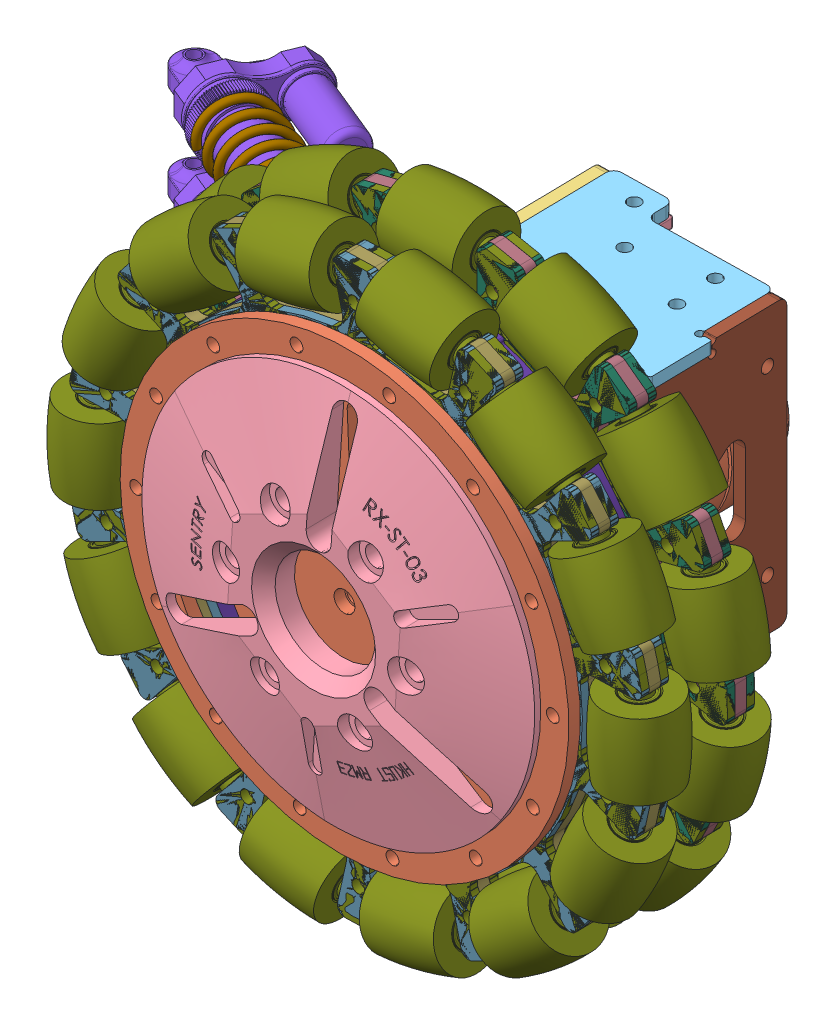
SolidWorks assembly 1.5GEN_sentry_suspension_module, configuration Default. Lengths in mm.
Overall size (247.79 229.92 117.48).
42 component instances, 23 part files, 105 mates.
Components (placement in the parent):
- 3508_standard_motor_mount1-1: 3508_standard_motor_mount1 [Default] at (120.0122 35.5003 50.6966) x (0.999831 0 -0.018366) z (0.018366 0 0.999831) size (47 66 13)
- M3508motor-1: M3508motor [默认] at (66.2746 27.3408 24.7382) x (0.383514 -0.923508 -0.007045) z (0.018366 0 0.999831) size (44.15 46.04 98.4)
- CF3mm_3508_housing_up-2: CF3mm_3508_housing_up [Default] at (60.787 36 124.2968) x (0 -1 0) z (-0.999831 0 0.018366) size (72 77 3)
- CNC_threaded_standard_part_L_shape_15x15x10x3-1: CNC_threaded_standard_part_L_shape_15x15x10x3 [Default] at (60.5115 69 109.2993) x (0.999831 0 -0.018366) z (-0.018366 0 -0.999831) size (15 15 10)
- CNC_threaded_standard_part_L_shape_15x15x10x3-2: CNC_threaded_standard_part_L_shape_15x15x10x3 [Default] at (59.5564 69 57.3081) x (0.999831 0 -0.018366) z (-0.018366 0 -0.999831) size (15 15 10)
- CF3mm_3508_housing_siding-1: CF3mm_3508_housing_siding [Default] at (82.7832 69 123.8927) x (-0.999831 0 0.018366) z (0 1 0) size (53 77 3)
- CNC_threaded_standard_part_L_shape_15x15x10x3-9: CNC_threaded_standard_part_L_shape_15x15x10x3 [Default] at (106.6771 3 63.4437) x (-0.999831 0 0.018366) z (-0.018366 0 -0.999831) size (15 15 10)
- CNC_threaded_standard_part_L_shape_15x15x10x3-10: CNC_threaded_standard_part_L_shape_15x15x10x3 [Default] at (59.3728 3 47.3097) x (0.999831 0 -0.018366) z (0.018366 0 0.999831) size (15 15 10)
- HITITECH_90mm_shock_absorber_SUM-4: HITITECH_90mm_shock_absorber_SUM [Default] at (1.775 57.362 93.1324) x (0.381638 -0.024239 -0.923994) z (-0.001153 -0.999668 0.025748) size (33.86 98.99 29.95) (flexible)
  - HITITECH_90mm_shock_absorber_rod-1: HITITECH_90mm_shock_absorber_rod [Default] at (-13.8895 -8.2919 48.3121) x (-0.999706 0.000547 0.024245) z (-0.024239 0.008761 -0.999668) size (9.5 43.16 9.6)
  - HITITECH_90mm_shock_absorber_cap-1: HITITECH_90mm_shock_absorber_cap [Default] at (4.5941 -7.8733 -1.1663) x (-0.024239 0.008761 -0.999668) z (0.999706 -0.000547 -0.024245) size (29.48 7.8 16.61)
  - HITITECH_90mm_shock_absorber_Base-1: HITITECH_90mm_shock_absorber_Base [Default] at (54.0743 -7.9124 17.3177) x (0.999706 -0.000547 -0.024245) z (0.024239 -0.008761 0.999668) size (30.67 56.88 16.99)
  - HITITECH_90mm_shock_absorber_SPRING_TEMPLATE-1: HITITECH_90mm_shock_absorber_SPRING_TEMPLATE [Default] at (20.0934 -6.7725 32.8265) x (-0.182655 -0.008459 0.983141) z (-0.983177 0.002344 -0.182642) size (17.85 56.5 20.09)
  - MATEING_ASSISTENT-1: MATEING_ASSISTENT [Default] at (20.071 -36.2888 32.5684) x (1 -0.00076 -0.000003) z (-0.000003 -0.008745 0.999962) size (10 3 10)
- CNC_threaded_standard_part_L_shape_15x15x10x3-11: CNC_threaded_standard_part_L_shape_15x15x10x3 [Default] at (107.5035 3 108.4361) x (-0.999831 0 0.018366) z (-0.018366 0 -0.999831) size (15 15 10)
- CF3mm_3508_housing_lower-3: CF3mm_3508_housing_lower [Default] at (110.7785 36 123.3784) x (0 -1 0) z (-0.999831 0 0.018366) size (72 76.78 3)
- CNC_threaded_standard_part_L_shape_15x15x10x3-12: CNC_threaded_standard_part_L_shape_15x15x10x3 [Default] at (60.3278 3 99.301) x (0.999831 0 -0.018366) z (0.018366 0 0.999831) size (15 15 10)
- CNC_threaded_standard_part_L_shape_15x15x10x3-13: CNC_threaded_standard_part_L_shape_15x15x10x3 [Default] at (107.5035 69 108.4361) x (0 -1 0) z (-0.018366 0 -0.999831) size (15 15 10)
- CNC_threaded_standard_part_L_shape_15x15x10x3-14: CNC_threaded_standard_part_L_shape_15x15x10x3 [Default] at (106.6771 69 63.4437) x (0 -1 0) z (-0.018366 0 -0.999831) size (15 15 10)
- HexRoll_omniwheel_for_SENTRY_1.5GEN-1: HexRoll_omniwheel_for_SENTRY_1.5GEN [Default] at (-49.9891 -57.0963 -138.1237) x (-0.47713 0.878789 0.008765) z (0.878641 0.477211 -0.01614) size (202.67 40 202.39) (flexible)
  - AL3mm_HexRoll_omniwheel_embed_board_w1-1: AL3mm_HexRoll_omniwheel_embed_board_w1 [Default] at (-308.948 305.7761 571.1073) x (0.925846 0 -0.377901) z (0.377901 0 0.925846) size (145 3 143.25)
  - AL3mm_HexRoll_omniwheel_embed_board_W2-1: AL3mm_HexRoll_omniwheel_embed_board_W2 [Default] at (-494.5908 284.7961 276.0744) x (0.959571 0 0.281468) z (-0.281468 0 0.959571) size (145 3 143.25)
  - CF2mm_HexRoll_omniwheel_roller_caps_w1-1: CF2mm_HexRoll_omniwheel_roller_caps_w1 [Default] at (82.1743 310.7861 312.095) x (0.925846 0 -0.377901) z (0.377901 0 0.925846) size (145 2 143.25)
  - CF2mm_HexRoll_omniwheel_roller_caps_w2-1: CF2mm_HexRoll_omniwheel_roller_caps_w2 [Default] at (-27.2933 284.8061 317.2692) x (0.959571 0 0.281468) z (-0.281468 0 0.959571) size (145 2 143.25)
  - HexRoll_omniwheel_roller_assemblys-1: HexRoll_omniwheel_roller_assemblys [Default] at (-208.6485 284.7861 634.0409) x (0.818343 0 -0.57473) z (0.57473 0 0.818343) size (153.68 40 153.68)
  - CF2mm_HexRoll_omniwheel_roller_caps_w1-2: CF2mm_HexRoll_omniwheel_roller_caps_w1 [Default] at (82.1743 305.7861 312.095) x (0.925846 0 -0.377901) z (0.377901 0 0.925846) size (145 2 143.25)
  - CF2mm_HexRoll_omniwheel_roller_caps_w2-2: CF2mm_HexRoll_omniwheel_roller_caps_w2 [Default] at (114.9142 289.8061 294.3775) x (0.818343 0 -0.57473) z (0.57473 0 0.818343) size (145 2 143.25)
  - 3D_ABS_ dual_omniwheel_system_infill-1: 3D_ABS_ dual_omniwheel_system_infill [Default] at (20.0429 257.4808 158.175) x (0.794197 0 -0.60766) z (0 1 0) size (113 112.12 13.98)
- 10x24x9_flat_thrust_bearing-1: 10x24x9_flat_thrust_bearing [Default] at (84.1921 36 118.916) x (-0.094331 0.995539 0.001733) z (0.018366 0 0.999831) size (24 24 9) (hidden)
- AL_3mm_washer_for_thrust-bearing-2: AL_3mm_washer_for_thrust-bearing [Default] at (84.137 36 115.9165) x (0.999807 -0.006986 -0.018366) z (0.018366 0 0.999831) size (42 42 3)
- CNC_上交菊花-1: CNC_上交菊花 [Default] at (84.3574 36 127.9145) x (-0.997601 0.06675 0.018325) z (0.066739 0.99777 -0.001226) size (56 10 49.97)
- CF3mm_菊花towheel_transmission-1: CF3mm_菊花towheel_transmission [Default] at (84.541 36 137.9128) x (-0.441003 0.897469 0.008101) z (0.018366 0 0.999831) size (112 112 3)
- CF3mm_3508_housing_siding-2: CF3mm_3508_housing_siding [Default] at (82.7832 0 123.8927) x (-0.999831 0 0.018366) z (0 1 0) size (53 77 3)
- 3mm固定座-3: 3mm固定座 [Default] at (57.7938 95.7194 124.6949) x (-0.018366 0 -0.999831) z (0 1 0) size (20 17.54 13)
- 3mm固定座-4: 3mm固定座 [Default] at (57.7938 71.7194 124.6949) x (-0.018366 0 -0.999831) z (0 1 0) size (20 17.54 13)
- HITITECH_90mm_shock_absorber_SUM-5: HITITECH_90mm_shock_absorber_SUM [Default] at (1.775 81.362 93.1324) x (0.381638 -0.024239 -0.923994) z (-0.001153 -0.999668 0.025748) size (34.14 98.99 29.95) (flexible)
  - HITITECH_90mm_shock_absorber_rod-1: HITITECH_90mm_shock_absorber_rod [Default] at (-13.8895 -8.2919 48.3121) x (-0.999706 0.000547 0.024245) z (-0.024239 0.008761 -0.999668) size (9.5 43.16 9.6)
  - HITITECH_90mm_shock_absorber_cap-1: HITITECH_90mm_shock_absorber_cap [Default] at (4.5941 -7.8733 -1.1663) x (-0.024239 0.008761 -0.999668) z (0.999706 -0.000547 -0.024245) size (29.48 7.8 16.61)
  - HITITECH_90mm_shock_absorber_Base-1: HITITECH_90mm_shock_absorber_Base [Default] at (54.0743 -7.9124 17.3177) x (0.999706 -0.000547 -0.024245) z (0.024239 -0.008761 0.999668) size (30.67 56.88 16.99)
  - HITITECH_90mm_shock_absorber_SPRING_TEMPLATE-1: HITITECH_90mm_shock_absorber_SPRING_TEMPLATE [Default] at (20.0934 -6.7725 32.8265) x (0.95392 0.0019 -0.300054) z (0.300059 -0.00857 0.953882) size (17.85 56.5 20.09)
  - MATEING_ASSISTENT-1: MATEING_ASSISTENT [Default] at (20.071 -36.2888 32.5684) x (1 -0.00076 -0.000003) z (-0.000003 -0.008745 0.999962) size (10 3 10)
- 3d_PETG_hexroll_omniwheel_outershell-1: 3d_PETG_hexroll_omniwheel_outershell [Default] at (84.5961 36 140.9123) x (0.997601 -0.06675 -0.018325) z (-0.066739 -0.99777 0.001226) size (98 10.06 98)
Mates (geometry in assembly coordinates):
- 同心1: concentric anti-aligned: cylinder of 3508_mount_flange_bearing-1 through (59.9995 81.1282 34.0361) axis (-0.013522 -0.681588 -0.731611) radius 10; cylinder of 3508_standard_motor_mount1-1 through (84.137 36 115.9165) axis (0.018366 0 0.999831) radius 21.015
- 重合1: coincident anti-aligned: plane of 3508_mount_flange_bearing-1 through (79.6528 88.4606 30.9033) normal (-0.013522 -0.681588 -0.731611); plane of 3508_standard_motor_mount1-1 through (84.137 36 115.9165) normal (0.018366 0 0.999831)
- 同心2: concentric aligned: cylinder of 3508_mount_flange-1 through (60.4081 101.7268 56.1464) axis (-0.013522 -0.681588 -0.731611) radius 30; cylinder of 3508_mount_flange_bearing-1 through (59.9995 81.1282 34.0361) axis (-0.013522 -0.681588 -0.731611) radius 10
- 同心3: concentric anti-aligned: cylinder of 3508_standard_motor_mount1-1 through (83.9882 36 107.8179) axis (0.018366 0 0.999831) radius 13.1; cylinder of M3508motor-1 through (83.3831 36 74.8734) axis (-0.018366 0 -0.999831) radius 21
- 重合3: coincident anti-aligned: plane of 3508_standard_motor_mount1-1 through (60.5482 3 111.2989) normal (-0.018366 0 -0.999831); plane of M3508motor-1 through (71.0464 36 111.1061) normal (0.018366 0 0.999831)
- 重合4: coincident anti-aligned: plane of 3508_mount_flange-1 through (63.1337 100.3879 50.5091) normal (-0.698286 -0.517267 0.494805); plane of M3508motor-1 through (89.1272 36.7071 118.0752) normal (0.706988 0.707107 -0.012987)
- 同心8: concentric anti-aligned: cylinder of 3508_mount_flange-1 through (62.9984 93.572 43.193) axis (-0.698286 -0.517267 0.494805) radius 1.5; cylinder of M3508motor-1 through (87.1899 38.8284 128.1125) axis (0.706988 0.707107 -0.012987) radius 1.25
- 同心9: concentric anti-aligned: cylinder of 3508_standard_motor_mount1-1 through (60.6676 21 117.7978) axis (-0.999831 0 0.018366) radius 2.1; cylinder of AL3mm_3508_housing_up-2 through (57.6681 21 117.8529) axis (0.999831 0 -0.018366) radius 2.6
- 同心10: concentric anti-aligned: cylinder of 3508_standard_motor_mount1-1 through (60.6676 51 117.7978) axis (-0.999831 0 0.018366) radius 2.1; cylinder of AL3mm_3508_housing_up-2 through (57.6681 51 117.8529) axis (0.999831 0 -0.018366) radius 2.6
- 重合5: coincident anti-aligned: plane of 3508_standard_motor_mount1-1 through (60.787 3 124.2968) normal (-0.999831 0 0.018366); plane of AL3mm_3508_housing_up-2 through (60.787 36 124.2968) normal (0.999831 0 -0.018366)
- 同心11: concentric aligned: cylinder of AL3mm_3508_housing_up-2 through (67.4185 59 104.1716) axis (-0.999831 0 0.018366) radius 1.6; cylinder of CNC_threaded_standard_part_L_shape_15x15x10x3-1 through (65.4188 59 104.2083) axis (-0.999831 0 0.018366) radius 1.6
- 重合6: coincident anti-aligned: plane of AL3mm_3508_housing_up-2 through (60.787 36 124.2968) normal (0.999831 0 -0.018366); plane of CNC_threaded_standard_part_L_shape_15x15x10x3-1 through (60.3278 54 99.301) normal (-0.999831 0 0.018366)
- 重合7: coincident anti-aligned: plane of AL3mm_3508_housing_up-2 through (60.787 36 124.2968) normal (0.999831 0 -0.018366); plane of CNC_threaded_standard_part_L_shape_15x15x10x3-2 through (59.3728 54 47.3097) normal (-0.999831 0 0.018366)
- 重合8: coincident aligned: plane of CNC_threaded_standard_part_L_shape_15x15x10x3-1 through (60.3278 69 99.301) normal (0 1 0); plane of CNC_threaded_standard_part_L_shape_15x15x10x3-2 through (59.3728 69 47.3097) normal (0 1 0)
- 同心13: concentric anti-aligned: cylinder of 3508_standard_motor_mount1-1 through (71.6657 69 117.5958) axis (0 1 0) radius 2.1; cylinder of AL3mm_3508_housing_siding-1 through (71.6657 72 117.5958) axis (0 -1 0) radius 2.6
- 同心14: concentric anti-aligned: cylinder of 3508_standard_motor_mount1-1 through (96.6615 69 117.1367) axis (0 1 0) radius 2.1; cylinder of AL3mm_3508_housing_siding-1 through (96.6615 72 117.1367) axis (0 -1 0) radius 2.6
- 重合9: coincident anti-aligned: plane of 3508_standard_motor_mount1-1 through (60.787 69 124.2968) normal (0 1 0); plane of AL3mm_3508_housing_siding-1 through (82.7832 69 123.8927) normal (0 -1 0)
- 平行1: parallel aligned: plane of AL3mm_3508_housing_siding-1 through (82.7832 72 123.8927) normal (0 1 0); plane of HITITECH_90mm_shock_absorber_SUM-1/HITITECH_90mm_shock_absorber_rod-1 through (-11.0401 90.0473 -33.0694) normal (0.000677 0.999674 0.025537)
- 平行2: parallel anti-aligned: plane of AL3mm_3508_housing_siding-1 through (82.7832 72 123.8927) normal (0 1 0); plane of HITITECH_90mm_shock_absorber_SUM-2/HITITECH_90mm_shock_absorber_rod-1 through (3.3061 110.5345 -19.2232) normal (-0.000677 -0.999674 -0.025537)
- 同心16: concentric: cylinder of AL3mm_3508_housing_siding-1 through (71.6657 72 117.5958) axis (0 -1 0) radius 2.6; cylinder of 双联3mm安装座B型-1 through (70.8172 111.8551 109.2453) axis (-0.00335 -0.985119 -0.171843) radius 2.55
- 同心17: concentric aligned: cylinder of AL3mm_3508_housing_siding-1 through (96.6615 72 117.1367) axis (0 -1 0) radius 2.6; cylinder of 双联3mm安装座B型-1 through (95.813 111.8499 108.7882) axis (-0.00335 -0.985119 -0.171843) radius 2.55
- 同心18: concentric anti-aligned: cylinder of M3508motor-1 through (83.1535 36 62.3755) axis (0.018366 0 0.999831) radius 20.98; cylinder of 3dprint_motorMountLight-3 through (84.1177 36 114.8667) axis (-0.018366 0 -0.999831) radius 13
- 平行6: parallel aligned: plane of AL3mm_3508_housing_up-2 through (57.7875 36 124.3519) normal (-0.999831 0 0.018366); plane of 3dprint_motorMountLight-3 through (51.1864 36 64.463) normal (-0.999831 0 0.018366)
- 重合16: coincident aligned: plane of 3508_standard_motor_mount1-1 through (60.5482 3 111.2989) normal (-0.018366 0 -0.999831); plane of 3dprint_motorMountLight-3 through (84.0442 36 110.8673) normal (-0.018366 0 -0.999831)
- 同心19: concentric anti-aligned: cylinder of AL3mm_3508_housing_siding-1 through (93.7303 69 93.6865) axis (0 1 0) radius 1.6; cylinder of 3mm固定座-2 through (93.7303 75 93.6865) axis (0 -1 0) radius 1.6
- 同心20: concentric anti-aligned: cylinder of AL3mm_3508_housing_siding-1 through (93.5467 69 83.6882) axis (0 1 0) radius 1.6; cylinder of 3mm固定座-2 through (93.5467 75 83.6882) axis (0 -1 0) radius 1.6
- 同心21: concentric anti-aligned: cylinder of AL3mm_3508_housing_siding-1 through (73.7337 69 94.0539) axis (0 1 0) radius 1.6; cylinder of 3mm固定座-1 through (73.7337 75 94.0539) axis (0 -1 0) radius 1.6
- 同心22: concentric anti-aligned: cylinder of AL3mm_3508_housing_siding-1 through (73.55 69 84.0556) axis (0 1 0) radius 1.6; cylinder of 3mm固定座-1 through (73.55 75 84.0556) axis (0 -1 0) radius 1.6
- 重合17: coincident anti-aligned: plane of AL3mm_3508_housing_siding-1 through (82.7832 72 123.8927) normal (0 1 0); plane of 3mm固定座-1 through (25.2814 72 54.594) normal (0 -1 0)
- 重合18: coincident anti-aligned: plane of AL3mm_3508_housing_siding-1 through (82.7832 72 123.8927) normal (0 1 0); plane of 3mm固定座-2 through (45.278 72 54.2267) normal (0 -1 0)
- 同心24: concentric aligned: cylinder of 3508_standard_motor_mount1-1 through (71.7087 48.3744 113.0943) axis (0.018366 0 0.999831) radius 3.8; cylinder of M3508motor-1 through (71.672 48.3744 111.0946) axis (0.018366 0 0.999831) radius 1.65
- 同心32: concentric anti-aligned: cylinder of 3508_standard_motor_mount1-1 through (96.6625 3 117.1446) axis (0 -1 0) radius 2.1; cylinder of AL3mm_3508_housing_lower-1 through (96.6625 0 117.1446) axis (0 1 0) radius 2.6
- 重合21: coincident aligned: plane of AL3mm_3508_housing_up-2 through (57.7875 36 124.3519) normal (-0.999831 0 0.018366); plane of AL3mm_3508_housing_lower-1 through (57.7885 0 124.3597) normal (-0.999831 0 0.018366)
- 重合22: coincident anti-aligned: plane of AL3mm_3508_housing_up-2 through (57.7875 3 124.3519) normal (0 -1 0); plane of AL3mm_3508_housing_lower-1 through (85.7838 3 123.8455) normal (0 1 0)
- 同心35: concentric: cylinder of AL3mm_3508_housing_lower-1 through (99.4604 10 78.8867) axis (0 -1 0) radius 1.6; cylinder of CNC_threaded_standard_part_L_shape_15x15x10x3-9 through (96.5869 8 58.6282) axis (0 -1 0) radius 1.6
- 重合23: coincident: plane of AL3mm_3508_housing_lower-1 through (85.7838 3 123.8455) normal (0 1 0); plane of CNC_threaded_standard_part_L_shape_15x15x10x3-9 through (106.4934 3 53.4454) normal (0 -1 0)
- 同心39: concentric aligned: cylinder of AL3mm_3508_housing_lower-1 through (67.4658 10 79.4744) axis (0 -1 0) radius 1.6; cylinder of CNC_threaded_standard_part_L_shape_15x15x10x3-10 through (69.4629 8 52.1252) axis (0 -1 0) radius 1.6
- 重合24: coincident anti-aligned: plane of AL3mm_3508_housing_up-2 through (60.787 36 124.2968) normal (0.999831 0 -0.018366); plane of CNC_threaded_standard_part_L_shape_15x15x10x3-10 through (59.5564 18 57.3081) normal (-0.999831 0 0.018366)
- 重合25: coincident anti-aligned: plane of AL3mm_3508_housing_lower-1 through (85.7838 3 123.8455) normal (0 1 0); plane of CNC_threaded_standard_part_L_shape_15x15x10x3-10 through (59.5564 3 57.3081) normal (0 -1 0)
- 同心52: concentric anti-aligned: cylinder of AL3mm_3508_housing_lower-1 through (99.914 0 103.5826) axis (0 1 0) radius 1.6; cylinder of CNC_threaded_standard_part_L_shape_15x15x10x3-11 through (97.4134 8 103.6206) axis (0 -1 0) radius 1.6
- 重合31: coincident anti-aligned: plane of AL3mm_3508_housing_lower-1 through (85.7838 3 123.8455) normal (0 1 0); plane of CNC_threaded_standard_part_L_shape_15x15x10x3-11 through (107.3199 3 98.4378) normal (0 -1 0)
- 重合32: coincident aligned: plane of AL3mm_3508_housing_lower-1 through (107.7801 0 123.4414) normal (0.999831 0 -0.018366); plane of CNC_threaded_standard_part_L_shape_15x15x10x3-11 through (107.3199 18 98.4378) normal (0.999831 0 -0.018366)
- 同心53: concentric anti-aligned: cylinder of CNC_threaded_standard_part_L_shape_15x15x10x3-11 through (102.4126 13 103.5287) axis (0.999831 0 -0.018366) radius 1.6; cylinder of AL3mm_3508_housing_upper-3 through (117.41 13 103.2533) axis (-0.999831 0 0.018366) radius 1.6
- 同心54: concentric anti-aligned: cylinder of CNC_threaded_standard_part_L_shape_15x15x10x3-9 through (101.5861 13 58.5363) axis (0.999831 0 -0.018366) radius 1.6; cylinder of AL3mm_3508_housing_upper-3 through (109.5847 13 58.3894) axis (-0.999831 0 0.018366) radius 1.6
- 重合33: coincident anti-aligned: plane of 3508_standard_motor_mount1-1 through (107.779 3 123.4335) normal (0.999831 0 -0.018366); plane of AL3mm_3508_housing_upper-3 through (107.779 36 123.4335) normal (-0.999831 0 0.018366)
- 同心57: concentric anti-aligned: cylinder of AL3mm_3508_housing_lower-1 through (67.9194 0 104.1703) axis (0 1 0) radius 1.6; cylinder of CNC_threaded_standard_part_L_shape_15x15x10x3-12 through (70.4179 8 104.1165) axis (0 -1 0) radius 1.6
- 重合35: coincident anti-aligned: plane of AL3mm_3508_housing_up-2 through (60.787 36 124.2968) normal (0.999831 0 -0.018366); plane of CNC_threaded_standard_part_L_shape_15x15x10x3-12 through (60.5115 18 109.2993) normal (-0.999831 0 0.018366)
- 重合36: coincident anti-aligned: plane of AL3mm_3508_housing_lower-1 through (85.7838 3 123.8455) normal (0 1 0); plane of CNC_threaded_standard_part_L_shape_15x15x10x3-12 through (60.5115 3 109.2993) normal (0 -1 0)
- 重合37: coincident anti-aligned: plane of AL3mm_3508_housing_upper-3 through (107.779 36 123.4335) normal (-0.999831 0 0.018366); plane of CNC_threaded_standard_part_L_shape_15x15x10x3-14 through (106.4934 69 53.4454) normal (0.999831 0 -0.018366)
- 重合38: coincident anti-aligned: plane of AL3mm_3508_housing_siding-1 through (82.7832 69 123.8927) normal (0 -1 0); plane of CNC_threaded_standard_part_L_shape_15x15x10x3-14 through (91.4959 69 53.7208) normal (0 1 0)
- 同心63: concentric anti-aligned: cylinder of AL3mm_3508_housing_siding-1 through (97.4134 72 103.6206) axis (0 -1 0) radius 1.6; cylinder of CNC_threaded_standard_part_L_shape_15x15x10x3-13 through (97.4134 64 103.6206) axis (0 1 0) radius 1.6
- 重合39: coincident anti-aligned: plane of AL3mm_3508_housing_upper-3 through (107.779 36 123.4335) normal (-0.999831 0 0.018366); plane of CNC_threaded_standard_part_L_shape_15x15x10x3-13 through (107.3199 69 98.4378) normal (0.999831 0 -0.018366)
- 重合40: coincident anti-aligned: plane of AL3mm_3508_housing_siding-1 through (82.7832 69 123.8927) normal (0 -1 0); plane of CNC_threaded_standard_part_L_shape_15x15x10x3-13 through (92.3224 69 98.7133) normal (0 1 0)
- 距离3: distance = 4 mm anti-aligned: plane of HexRoll_omniwheel_roller_assemblys-1 through (60.2864 95.5925 49.5619) normal (0.013522 0.681588 0.731611); plane of 3508_mount_flange-1 through (60.3405 98.3188 52.4883) normal (-0.013522 -0.681588 -0.731611)
- 同心64: concentric anti-aligned: cylinder of 3508_mount_flange-1 through (60.4081 101.7268 56.1464) axis (-0.013522 -0.681588 -0.731611) radius 30; cylinder of HexRoll_omniwheel_for_SENTRY_1.5GEN-1/CF2mm_HexRoll_omniwheel_roller_caps_w1-1 through (84.5043 36 135.9131) axis (0.018366 0 0.999831) radius 49
- 同心65: concentric anti-aligned: cylinder of M3508motor-1 through (84.5456 36 138.1627) axis (0.018366 0 0.999831) radius 5; cylinder of 10x24x9_flat_thrust_bearing-1 through (84.3574 36 127.9145) axis (-0.018366 0 -0.999831) radius 5
- 同心66: concentric anti-aligned: cylinder of M3508motor-1 through (84.5456 36 138.1627) axis (0.018366 0 0.999831) radius 5; cylinder of AL_3mm_washer_for_thrust-bearing-2 through (84.1921 36 118.916) axis (-0.018366 0 -0.999831) radius 9
- 重合46: coincident anti-aligned: plane of 3508_standard_motor_mount1-1 through (84.137 36 115.9165) normal (0.018366 0 0.999831); plane of AL_3mm_washer_for_thrust-bearing-2 through (84.137 36 115.9165) normal (-0.018366 0 -0.999831)
- 重合47: coincident anti-aligned: plane of 10x24x9_flat_thrust_bearing-1 through (84.1921 36 118.916) normal (-0.018366 0 -0.999831); plane of AL_3mm_washer_for_thrust-bearing-2 through (84.1921 36 118.916) normal (0.018366 0 0.999831)
- 同心67: concentric anti-aligned: cylinder of M3508motor-1 through (84.5456 36 138.1627) axis (0.018366 0 0.999831) radius 5; cylinder of CNC_上交菊花-1 through (84.541 36 137.9128) axis (-0.018366 0 -0.999831) radius 5
- 重合48: coincident anti-aligned: plane of 10x24x9_flat_thrust_bearing-1 through (84.3574 36 127.9145) normal (0.018366 0 0.999831); plane of CNC_上交菊花-1 through (84.3574 36 127.9145) normal (-0.018366 0 -0.999831)
- 同心68: concentric anti-aligned: cylinder of M3508motor-1 through (84.5456 36 138.1627) axis (0.018366 0 0.999831) radius 2.1; cylinder of HexRoll_omniwheel_for_SENTRY_1.5GEN-1/3D_ABS_ dual_omniwheel_system_infill-1 through (84.4125 36 130.914) axis (-0.018366 0 -0.999831) radius 49
- 同心69: concentric anti-aligned: cylinder of M3508motor-1 through (84.5456 36 138.1627) axis (0.018366 0 0.999831) radius 2.1; cylinder of CF4mm_菊花towheel_transmission-1 through (84.5961 36 140.9123) axis (-0.018366 0 -0.999831) radius 2.6
- 同心70: concentric anti-aligned: cylinder of HexRoll_omniwheel_for_SENTRY_1.5GEN-1/CF2mm_HexRoll_omniwheel_roller_caps_w1-1 through (52.3962 -4.9133 135.5027) axis (0.018366 0 0.999831) radius 1.6; cylinder of CF4mm_菊花towheel_transmission-1 through (52.5064 -4.9133 141.5017) axis (-0.018366 0 -0.999831) radius 1.6
- 重合49: coincident anti-aligned: plane of CNC_上交菊花-1 through (84.541 36 137.9128) normal (0.018366 0 0.999831); plane of CF4mm_菊花towheel_transmission-1 through (84.541 36 137.9128) normal (-0.018366 0 -0.999831)
- 同心71: concentric aligned: cylinder of CNC_上交菊花-1 through (72.0176 17.3088 138.1428) axis (-0.018366 0 -0.999831) radius 2.5; cylinder of CF4mm_菊花towheel_transmission-1 through (72.0727 17.3088 141.1423) axis (-0.018366 0 -0.999831) radius 2.5
- 同心72: concentric aligned: cylinder of CF3mm_菊花towheel_transmission-1 through (84.5961 36 140.9123) axis (-0.018366 0 -0.999831) radius 56; cylinder of CF4mm_菊花towheel_transmission_spacer-1 through (84.541 36 137.9128) axis (-0.018366 0 -0.999831) radius 56
- 同心73: concentric aligned: cylinder of CF3mm_菊花towheel_transmission-1 through (96.5704 -14.6021 140.6923) axis (-0.018366 0 -0.999831) radius 1.6; cylinder of CF4mm_菊花towheel_transmission_spacer-1 through (76.508 -15.3756 138.0603) axis (-0.018366 0 -0.999831) radius 1.6
- 重合50: coincident anti-aligned: plane of CF3mm_菊花towheel_transmission-1 through (84.541 36 137.9128) normal (-0.018366 0 -0.999831); plane of CF4mm_菊花towheel_transmission_spacer-1 through (84.541 36 137.9128) normal (0.018366 0 0.999831)
- 重合51: coincident anti-aligned: plane of HexRoll_omniwheel_for_SENTRY_1.5GEN-1/CF2mm_HexRoll_omniwheel_roller_caps_w1-1 through (84.541 36 137.9128) normal (0.018366 0 0.999831); plane of CF4mm_菊花towheel_transmission_spacer-1 through (84.4676 36 133.9135) normal (-0.018366 0 -0.999831)
- 重合52: coincident anti-aligned: plane of AL3mm_3508_housing_lower-1 through (85.7838 0 123.8455) normal (0 -1 0)
- 同心74: concentric aligned: cylinder of CNC_threaded_standard_part_L_shape_15x15x10x3-2 through (69.4629 64 52.1252) axis (0 1 0) radius 1.6; cylinder of AL3mm_3508_housing_siding-1 through (69.4629 69 52.1252) axis (0 1 0) radius 1.6
- 同心75: concentric anti-aligned: cylinder of AL3mm_3508_housing_upper-3 through (109.5847 59 58.3894) axis (-0.999831 0 0.018366) radius 1.6; cylinder of CNC_threaded_standard_part_L_shape_15x15x10x3-14 through (101.5861 59 58.5363) axis (0.999831 0 -0.018366) radius 1.6
- 同心76: concentric anti-aligned: cylinder of AL3mm_3508_housing_siding-1 through (96.5869 72 58.6282) axis (0 -1 0) radius 1.6; cylinder of CNC_threaded_standard_part_L_shape_15x15x10x3-14 through (96.5869 64 58.6282) axis (0 1 0) radius 1.6
- 同心77: concentric anti-aligned: cylinder of AL3mm_3508_housing_upper-3 through (117.41 59 103.2533) axis (-0.999831 0 0.018366) radius 1.6; cylinder of CNC_threaded_standard_part_L_shape_15x15x10x3-13 through (102.4126 59 103.5287) axis (0.999831 0 -0.018366) radius 1.6
- 同心78: concentric aligned: cylinder of AL3mm_3508_housing_up-2 through (59.4646 13 52.3089) axis (-0.999831 0 0.018366) radius 1.6; cylinder of CNC_threaded_standard_part_L_shape_15x15x10x3-10 through (64.4638 13 52.2171) axis (-0.999831 0 0.018366) radius 1.6
- 同心79: concentric anti-aligned: cylinder of CNC_threaded_standard_part_L_shape_15x15x10x3-9 through (101.5861 13 58.5363) axis (0.999831 0 -0.018366) radius 1.6; cylinder of AL3mm_3508_housing_upper-3 through (109.5847 13 58.3894) axis (-0.999831 0 0.018366) radius 1.6
- 平行7: parallel aligned: plane of CNC_threaded_standard_part_L_shape_15x15x10x3-9 through (106.4934 3 53.4454) normal (0 -1 0); plane of AL3mm_3508_housing_upper-3 through (107.779 0 123.4335) normal (0 -1 0)
- 重合54: coincident anti-aligned: plane of CNC_threaded_standard_part_L_shape_15x15x10x3-9 through (106.4934 18 53.4454) normal (0.999831 0 -0.018366); plane of AL3mm_3508_housing_upper-3 through (107.779 36 123.4335) normal (-0.999831 0 0.018366)
- 同心80: concentric anti-aligned: cylinder of CNC_threaded_standard_part_L_shape_15x15x10x3-11 through (102.4126 13 103.5287) axis (0.999831 0 -0.018366) radius 1.6; cylinder of AL3mm_3508_housing_upper-3 through (117.41 13 103.2533) axis (-0.999831 0 0.018366) radius 1.6
- 重合55: coincident aligned: plane of CNC_threaded_standard_part_L_shape_15x15x10x3-11 through (107.3199 3 98.4378) normal (0 -1 0); plane of AL3mm_3508_housing_upper-3 through (107.779 3 123.4335) normal (0 -1 0)
- 重合56: coincident anti-aligned: plane of CNC_threaded_standard_part_L_shape_15x15x10x3-11 through (107.3199 18 98.4378) normal (0.999831 0 -0.018366); plane of AL3mm_3508_housing_upper-3 through (107.779 36 123.4335) normal (-0.999831 0 0.018366)
- 同心81: concentric aligned: cylinder of CNC_threaded_standard_part_L_shape_15x15x10x3-12 through (70.4179 8 104.1165) axis (0 -1 0) radius 1.6; cylinder of AL3mm_3508_housing_siding-2 through (70.4179 3 104.1165) axis (0 -1 0) radius 1.6
- 同心82: concentric anti-aligned: cylinder of CNC_threaded_standard_part_L_shape_15x15x10x3-10 through (69.4629 8 52.1252) axis (0 -1 0) radius 1.6; cylinder of AL3mm_3508_housing_siding-2 through (69.4629 0 52.1252) axis (0 1 0) radius 1.6
- 同心83: concentric aligned: cylinder of CNC_threaded_standard_part_L_shape_15x15x10x3-9 through (96.5869 8 58.6282) axis (0 -1 0) radius 1.6; cylinder of AL3mm_3508_housing_siding-2 through (96.5869 3 58.6282) axis (0 -1 0) radius 1.6
- 重合57: coincident anti-aligned: plane of CNC_threaded_standard_part_L_shape_15x15x10x3-9 through (106.4934 3 53.4454) normal (0 -1 0); plane of AL3mm_3508_housing_siding-2 through (82.7832 3 123.8927) normal (0 1 0)
- 同心84: concentric anti-aligned: cylinder of AL3mm_3508_housing_up-2 through (67.2348 48 94.1732) axis (-0.999831 0 0.018366) radius 1.6; cylinder of 3mm固定座-3 through (54.237 48 94.412) axis (0.999831 0 -0.018366) radius 1.6
- 同心85: concentric anti-aligned: cylinder of AL3mm_3508_housing_up-2 through (67.0511 48 84.1749) axis (-0.999831 0 0.018366) radius 1.6; cylinder of 3mm固定座-3 through (54.0533 48 84.4137) axis (0.999831 0 -0.018366) radius 1.6
- 重合58: coincident anti-aligned: plane of AL3mm_3508_housing_up-2 through (57.7875 36 124.3519) normal (-0.999831 0 0.018366); plane of 3mm固定座-3 through (57.7938 95.7194 124.6949) normal (0.999831 0 -0.018366)
- 同心86: concentric anti-aligned: cylinder of AL3mm_3508_housing_up-2 through (67.2348 24 94.1732) axis (-0.999831 0 0.018366) radius 1.6; cylinder of 3mm固定座-4 through (54.237 24 94.412) axis (0.999831 0 -0.018366) radius 1.6
- 同心87: concentric anti-aligned: cylinder of AL3mm_3508_housing_up-2 through (67.0511 24 84.1749) axis (-0.999831 0 0.018366) radius 1.6; cylinder of 3mm固定座-4 through (54.0533 24 84.4137) axis (0.999831 0 -0.018366) radius 1.6
- 重合59: coincident anti-aligned: plane of AL3mm_3508_housing_up-2 through (57.7875 36 124.3519) normal (-0.999831 0 0.018366); plane of 3mm固定座-4 through (57.7938 71.7194 124.6949) normal (0.999831 0 -0.018366)
- 同心88: concentric aligned: cylinder of HITITECH_90mm_shock_absorber_SUM-4/HITITECH_90mm_shock_absorber_rod-1 through (43.8469 30.5 89.602) axis (0 -1 0) radius 1.5686; cylinder of 3mm固定座-3 through (43.8469 54.5 89.602) axis (0 -1 0) radius 1.5
- 同心89: concentric: cylinder of HITITECH_90mm_shock_absorber_SUM-3/HITITECH_90mm_shock_absorber_rod-1 through (43.8469 52.5 89.602) axis (0 -1 0) radius 1.5686; cylinder of 3mm固定座-4 through (43.8469 17.5 89.602) axis (0 1 0) radius 1.5
- 宽度1: width: plane of 3mm固定座-3 through (54.4941 52.2 108.4096) normal (0 -1 0); plane of HITITECH_90mm_shock_absorber_SUM-3/HITITECH_90mm_shock_absorber_rod-1 through (54.4941 43.8 108.4096) normal (0 1 0); plane of 3mm固定座-3 through (43.8469 49.5 89.602) normal (0 1 0); plane of HITITECH_90mm_shock_absorber_SUM-3/HITITECH_90mm_shock_absorber_rod-1 through (43.8469 42.5 89.602) normal (0 -1 0)
- 宽度2: width anti-aligned: plane of 3mm固定座-4 through (54.4941 28.2 108.4096) normal (0 -1 0); plane of HITITECH_90mm_shock_absorber_SUM-4/HITITECH_90mm_shock_absorber_rod-1 through (54.4941 19.8 108.4096) normal (0 1 0); plane of 3mm固定座-4 through (43.8469 20.5 89.602) normal (0 -1 0); plane of HITITECH_90mm_shock_absorber_SUM-4/HITITECH_90mm_shock_absorber_rod-1 through (43.8469 27.5 89.602) normal (0 1 0)
- 同心90: concentric aligned: cylinder of 3mm固定座-3 through (43.8469 54.5 89.602) axis (0 -1 0) radius 1.5; cylinder of HITITECH_90mm_shock_absorber_SUM-5/HITITECH_90mm_shock_absorber_rod-1 through (43.8469 54.5 89.602) axis (0 -1 0) radius 1.5686
- 同心93: concentric aligned: cylinder of HITITECH_90mm_shock_absorber_SUM-4/HITITECH_90mm_shock_absorber_Base-1 through (-39.2151 30.25 55.3688) axis (0 -1 0) radius 1.61; cylinder of HITITECH_90mm_shock_absorber_SUM-5/HITITECH_90mm_shock_absorber_Base-1 through (-39.2151 54.25 55.3688) axis (0 -1 0) radius 1.61
- 宽度3: width anti-aligned: plane of 3mm固定座-3 through (54.4941 43.8 108.4096) normal (0 1 0); plane of HITITECH_90mm_shock_absorber_SUM-5/HITITECH_90mm_shock_absorber_rod-1 through (54.4941 52.2 108.4096) normal (0 -1 0); plane of 3mm固定座-3 through (43.8469 44.5 89.602) normal (0 -1 0); plane of HITITECH_90mm_shock_absorber_SUM-5/HITITECH_90mm_shock_absorber_rod-1 through (43.8469 51.5 89.602) normal (0 1 0)
- 同心94: concentric anti-aligned: cylinder of HexRoll_omniwheel_for_SENTRY_1.5GEN-1/CF2mm_HexRoll_omniwheel_roller_caps_w1-1 through (96.4602 -14.6021 134.6933) axis (0.018366 0 0.999831) radius 1.6; cylinder of CF4mm_菊花towheel_transmission-1 through (96.5704 -14.6021 140.6923) axis (-0.018366 0 -0.999831) radius 1.6
- 重合60: coincident anti-aligned: plane of HexRoll_omniwheel_for_SENTRY_1.5GEN-1/CF2mm_HexRoll_omniwheel_roller_caps_w1-1 through (84.541 36 137.9128) normal (0.018366 0 0.999831); plane of CF4mm_菊花towheel_transmission-1 through (84.541 36 137.9128) normal (-0.018366 0 -0.999831)
- 重合61: coincident anti-aligned: plane of CNC_threaded_standard_part_L_shape_15x15x10x3-12 through (60.5115 3 109.2993) normal (0 -1 0); plane of AL3mm_3508_housing_siding-2 through (82.7832 3 123.8927) normal (0 1 0)
- 同心95: concentric anti-aligned: cylinder of CF4mm_菊花towheel_transmission-1 through (84.5961 36 140.9123) axis (-0.018366 0 -0.999831) radius 56; cylinder of 3d_PETG_hexroll_omniwheel_outershell-1 through (84.5594 36 138.9126) axis (0.018366 0 0.999831) radius 12.5
- 重合62: coincident anti-aligned: plane of CF4mm_菊花towheel_transmission-1 through (84.5961 36 140.9123) normal (0.018366 0 0.999831); plane of 3d_PETG_hexroll_omniwheel_outershell-1 through (84.5961 36 140.9123) normal (-0.018366 0 -0.999831)
- 重合63: coincident anti-aligned: circle of CNC_上交菊花-1; cylinder of 3d_PETG_hexroll_omniwheel_outershell-1 through (72.2563 17.3088 151.1406) axis (-0.018366 0 -0.999831) radius 2.5
